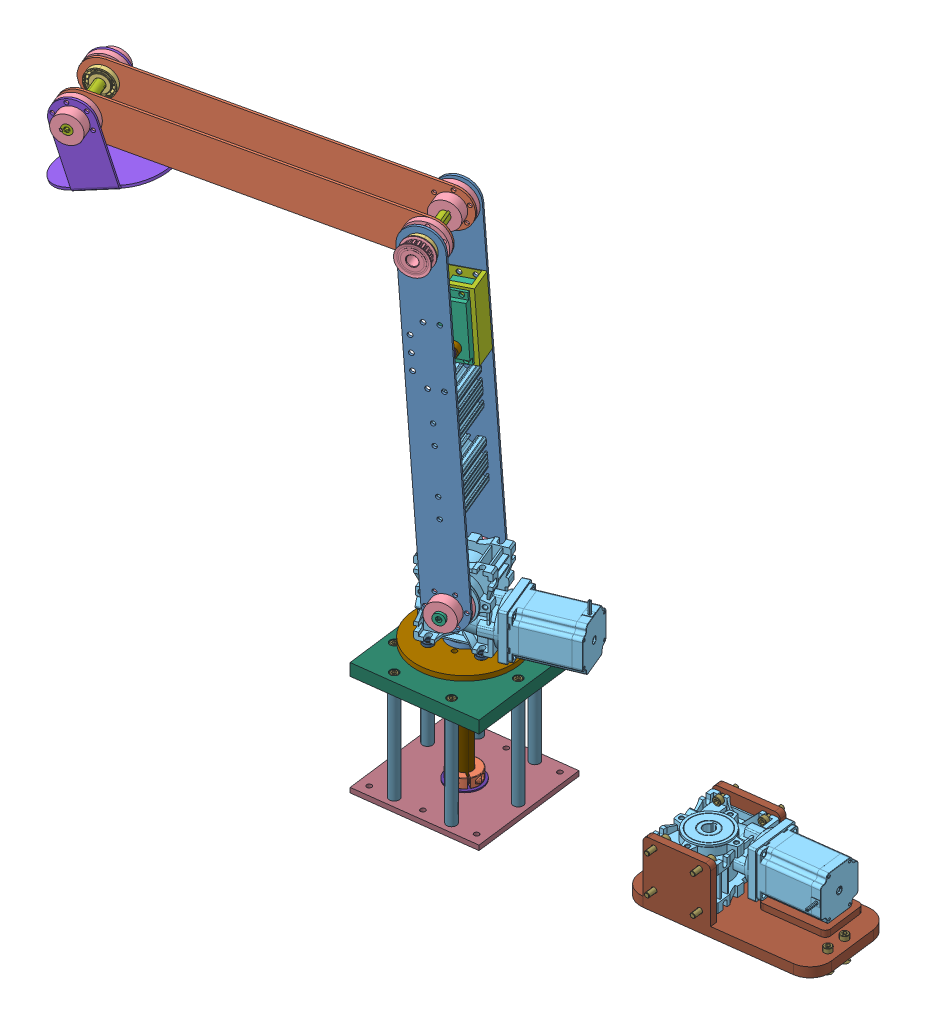
SolidWorks assembly Arm Assembly, configuration Default. Lengths in mm.
Overall size (892.51 782.73 345.65).
75 component instances, 30 part files, 141 mates.
Components (placement in the parent):
- Link 2-1: Link 2 [Default] at (1.4555 309.9129 324.2552) x (-0.057253 0.998075 0.023842) z (0.384426 0 0.923156) size (457.2 50.8 3.17)
- Link 3-1: Link 3 [Default] at (-14.0638 739.0935 409.0348) x (-0.91364 0.143211 0.380463) z (0.384426 0 0.923156) size (406.4 50.8 3.17)
- Flanged Bearing-1: Flanged Bearing [Default] at (-362.4163 764.8812 497.4483) x (0.923156 0 -0.384426) z (0.384426 0 0.923156) size (38.1 38.1 12.7)
- Keyed hub-1: Keyed hub [Default] at (9.2342 308.3376 408.8803) x (0.510272 -0.833349 -0.21249) z (-0.769311 -0.552748 0.320361) size (50.8 25.4 50.8)
- Link 2-2: Link 2 [Default] at (35.6886 309.9129 406.4623) x (-0.057253 0.998075 0.023842) z (0.384426 0 0.923156) size (457.2 50.8 3.17)
- Link 3-2: Link 3 [Default] at (-35.4177 739.0935 357.7558) x (-0.91364 0.143211 0.380463) z (0.384426 0 0.923156) size (406.4 50.8 3.17)
- Flanged Bearing-2: Flanged Bearing [Default] at (-9.7324 713.9553 428.8986) x (-0.878921 0.30584 0.366005) z (0.384426 0 0.923156) size (38.1 38.1 12.7)
- Flanged Bearing-3: Flanged Bearing [Default] at (-342.3416 764.8812 545.6555) x (-0.852745 -0.383049 0.355105) z (-0.384426 0 -0.923156) size (38.1 38.1 12.7)
- Keyed hub-2: Keyed hub [Default] at (-41.8271 713.9553 351.8267) x (0.725133 -0.618871 -0.301964) z (-0.571314 -0.785493 0.23791) size (50.8 25.4 50.8)
- Keyed hub-3: Keyed hub [Default] at (-17.6756 308.3376 344.2594) x (-0.510272 0.833349 0.21249) z (-0.769311 -0.552748 0.320361) size (50.8 25.4 50.8)
- Keyed hub-4: Keyed hub [Default] at (-13.1499 713.9553 420.6917) x (-0.725133 0.618871 0.301964) z (-0.571314 -0.785493 0.23791) size (50.8 25.4 50.8)
- Flanged Bearing-4: Flanged Bearing [Default] at (-45.2446 713.9553 343.6198) x (0.850075 0.38995 -0.353993) z (-0.384426 0 -0.923156) size (38.1 38.1 12.7)
- Nema Stepper Motor-2: Nema Stepper Motor [Default] at (64.8327 289.3684 347.8143) x (0.923156 0 -0.384426) z (-0.384426 0 -0.923156) size (171.01 100.01 63.01)
- Keyed Drive Shaft-1: Keyed Drive Shaft [Default] at (-50.3021 308.1752 256.2107) x (0.510272 -0.833349 -0.21249) z (0.384426 0 0.923156) size (19.9 19.9 128.01)
- Keyed Shaft-1: Keyed Shaft [Default] at (-51.2311 713.9553 329.2439) x (0.725133 -0.618871 -0.301964) z (0.384426 0 0.923156) size (12.7 12.5 104.14)
- Link 4-1: Link 4 [Default] at (-352.9478 683.5388 522.7917) x (0.384426 0 0.923156) z (-0.879568 -0.303649 0.366275) size (90.37 102.6 133.86)
- Keyed hub-5: Keyed hub [Default] at (-365.122 764.8812 490.9509) x (0.280315 -0.952784 -0.11673) z (0.879568 0.303649 -0.366275) size (50.8 25.4 50.8)
- Keyed hub-6: Keyed hub [Default] at (-338.9241 764.8812 553.8623) x (-0.280315 0.952784 0.11673) z (0.879568 0.303649 -0.366275) size (50.8 25.4 50.8)
- Keyed Shaft-2: Keyed Shaft [Default] at (-325.2539 764.8812 586.6897) x (0.280315 -0.952784 -0.11673) z (-0.384426 0 -0.923156) size (12.7 12.5 104.14)
- Joint 2 Motor Plate-1: Joint 2 Motor Plate [Default] at (-4.244 240.9876 376.7854) x (0.927827 0 0.373012) z (-0.373012 0 0.927827) size (127 6.35 127)
- 4 mm M6 spacer-1: 4 mm M6 spacer [94669A162] at (29.9074 249.3376 388.5617) x (-0.888418 0 -0.459036) z (0 -1 0) size (13 13 4)
- 4 mm M6 spacer-2: 4 mm M6 spacer [94669A162] at (-19.943 249.3376 409.3207) x (0.999963 0 0.008554) z (0 -1 0) size (13 13 4)
- 4 mm M6 spacer-3: 4 mm M6 spacer [94669A162] at (11.455 249.3376 344.2502) x (1 0 0) z (0 -1 0) size (13 13 4)
- 4 mm M6 spacer-4: 4 mm M6 spacer [94669A162] at (-38.3955 249.3376 365.0092) x (1 0 0) z (0 -1 0) size (13 13 4)
- Motor Mount Joint 1 Assembly-1: Motor Mount Joint 1 Assembly [Default] at (255.7253 -1.2672 148.6448) x (0.992107 0 -0.125391) z (0.125391 0 0.992107) size (228.6 94.85 140.08)
  - Joint 1 Motor Holder Bracket-1: Joint 1 Motor Holder Bracket [Default] at (55.8829 79.1234 191.166) size (228.6 82.55 114.78)
  - Nema Stepper Motor-1: Nema Stepper Motor [Default] at (81.7887 128.4828 180.6968) x (1 0 0) z (0 1 0) size (171.01 100.01 63.01)
  - Flanged Bearing-1: Flanged Bearing [Default] at (6.9829 88.5722 199.666) x (0.99323 0 0.116162) z (0 -1 0) size (38.1 38.1 12.7)
  - socket head cap screw_am-7: socket head cap screw_am [B18.3.1M - 6 x 1.0 x 25 Hex SHCS -- 25NHX] at (-20.0631 152.4828 153.666) x (0 0 -1) z (0.990069 0.140585 0) size (31 10 10)
  - socket head cap screw_am-8: socket head cap screw_am [B18.3.1M - 6 x 1.0 x 25 Hex SHCS -- 25NHX] at (33.9369 152.4828 228.666) x (0 0 1) z (-1 0 0) size (31 10 10)
  - socket head cap screw_am-9: socket head cap screw_am [B18.3.1M - 6 x 1.0 x 25 Hex SHCS -- 25NHX] at (-20.0631 152.4828 228.666) x (0 0 1) z (0.381849 0.924225 0) size (31 10 10)
  - socket head cap screw_am-10: socket head cap screw_am [B18.3.1M - 6 x 1.0 x 25 Hex SHCS -- 25NHX] at (-20.0631 104.4828 153.666) x (0 0 -1) z (0.756248 0.654286 0) size (31 10 10)
  - socket head cap screw_am-11: socket head cap screw_am [B18.3.1M - 6 x 1.0 x 25 Hex SHCS -- 25NHX] at (33.9369 104.4828 150.5881) x (0 0 -1) z (0.923728 0.383049 0) size (31 10 10)
  - socket head cap screw_am-12: socket head cap screw_am [B18.3.1M - 6 x 1.0 x 25 Hex SHCS -- 25NHX] at (-45.7171 97.8234 212.366) x (0 -1 0) z (-0.546944 0 0.837169) size (31 10 10)
  - socket head cap screw_am-19: socket head cap screw_am [B18.3.1M - 6 x 1.0 x 25 Hex SHCS -- 25NHX] at (-45.7171 97.8234 186.966) x (0 -1 0) z (-0.546944 0 0.837169) size (31 10 10)
  - socket head cap screw_am-14: socket head cap screw_am [B18.3.1M - 6 x 1.0 x 25 Hex SHCS -- 25NHX] at (33.9369 152.4828 153.666) x (0 0 -1) z (0.923728 0.383049 0) size (31 10 10)
  - socket head cap screw_am-15: socket head cap screw_am [B18.3.1M - 6 x 1.0 x 25 Hex SHCS -- 25NHX] at (157.4829 97.8234 186.966) x (0 -1 0) z (-0.546944 0 0.837169) size (31 10 10)
  - socket head cap screw_am-16: socket head cap screw_am [B18.3.1M - 6 x 1.0 x 25 Hex SHCS -- 25NHX] at (-20.0631 104.4828 228.666) x (0 0 1) z (-1 0 0) size (31 10 10)
  - socket head cap screw_am-17: socket head cap screw_am [B18.3.1M - 6 x 1.0 x 25 Hex SHCS -- 25NHX] at (33.9369 104.4828 228.666) x (0 0 1) z (-1 0 0) size (31 10 10)
  - socket head cap screw_am-18: socket head cap screw_am [B18.3.1M - 6 x 1.0 x 25 Hex SHCS -- 25NHX] at (157.4829 97.8234 212.366) x (0 -1 0) z (-0.546944 0 0.837169) size (31 10 10)
- Joint 1 bottom plate-1: Joint 1 bottom plate [89155K113] at (-4.244 81.0311 376.7854) x (-0.125391 0 -0.992107) z (0.992107 0 -0.125391) size (152.4 6.35 152.4)
- Base post-1: Base post [8974K269] at (21.393 160.4061 309.54) x (-0.837169 0 -0.546944) z (0 -1 0) size (12.7 12.7 127)
- Base post-2: Base post [8974K269] at (-29.8811 160.4061 444.0308) x (-0.837169 0 -0.546944) z (0 -1 0) size (12.7 12.7 127)
- Base post-3: Base post [8974K269] at (37.3177 160.4061 435.5376) x (0.463623 0 0.886032) z (0 -1 0) size (12.7 12.7 127)
- Base post-4: Base post [8974K269] at (58.7548 160.4061 368.8231) x (-0.837169 0 -0.546944) z (0 -1 0) size (12.7 12.7 127)
- Base post-5: Base post [8974K269] at (-70.4278 160.4061 359.5483) x (-0.837169 0 -0.546944) z (0 -1 0) size (12.7 12.7 127)
- Base post-6: Base post [8974K269] at (-45.8058 160.4061 318.0332) x (-0.837169 0 -0.546944) z (0 -1 0) size (12.7 12.7 127)
- Base post-7: Base post [8974K269] at (-64.0579 160.4061 409.9473) x (-0.837169 0 -0.546944) z (0 -1 0) size (12.7 12.7 127)
- Joint 1 top plate-1: Joint 1 top plate [89155K143] at (-4.244 219.1436 376.7854) x (-0.125391 0 -0.992107) z (0.992107 0 -0.125391) size (152.4 15.88 152.4)
- Tapered-Roller Bearing-1: Tapered-Roller Bearing [5709K77] at (-4.244 223.5886 376.7854) x (1 0 0) z (0 -1 0) size (45.24 45.24 17.1)
- base Ball Bearing 0.75 in-1: base Ball Bearing 0.75 in [6384K367] at (-4.244 79.4436 376.7854) x (1 0 0) z (0 -1 0) size (44.45 44.45 14.27)
- keyed shaft 0.75 in bore 9 in-1: keyed shaft 0.75 in bore 9 in [Default] at (-4.244 140.9751 376.7854) x (0.927827 0 0.373012) z (0 -1 0) size (19.05 18.75 228.6)
- 0.75 in shaft hub-1: 0.75 in shaft hub [Default] at (-4.244 234.6376 376.7854) x (-0.927827 0 -0.373012) z (0 -1 0) size (63.5 63.5 19.49)
- Clamping Two-Piece Shaft Collar 0.75 in-1: Clamping Two-Piece Shaft Collar 0.75 in [6436K16] at (-4.244 92.1436 376.7854) x (0.845517 0 0.533948) z (0 1 0) size (38.06 38.1 12.77)
- T-slot Slider-1: T-slot Slider [5278N52] at (236.9979 67.7205 365.0672) x (-0.837169 0 -0.546944) z (0 1 0) size (10 9.8 4.82)
- T-slot Slider-2: T-slot Slider [5278N52] at (233.8129 65.4156 339.8677) x (-0.837169 0 -0.546944) z (0 1 0) size (10 9.8 4.82)
- T-slot Slider-3: T-slot Slider [5278N52] at (438.5941 68.7454 339.5877) x (-0.838988 0 -0.544149) z (0 1 0) size (10 9.8 4.82)
- T-slot Slider-4: T-slot Slider [5278N52] at (435.4091 66.889 314.3882) x (-0.837169 0 -0.546944) z (0 1 0) size (10 9.8 4.82)
- joint3pulley-1: joint3pulley [6495K752] at (-5.8985 713.9553 438.1053) x (0.86916 -0.336987 -0.36194) z (-0.384426 0 -0.923156) size (38.1 38.1 22.23)
- 8020tframeforjoint3-1: 8020tframeforjoint3 [47065T653] at (-23.5517 422.4176 348.5885) x (0.921379 0.062019 -0.383686) z (0.384426 0 0.923156) size (25.4 50.8 85.85)
- 8020tframeforjoint3-2: 8020tframeforjoint3 [47065T653] at (-28.285 504.9314 350.5596) x (0.921379 0.062019 -0.383686) z (0.384426 0 0.923156) size (25.4 50.8 85.85)
- 80 kg-1: 80 kg [Default] at (-47.5369 625.3222 348.9217) x (0.057253 -0.998075 -0.023842) z (-0.921379 -0.062019 0.383686) size (82 48 30)
- servobracket_80kg-1: servobracket_80kg [Default] at (-37.0502 593.4851 343.7293) x (0.057253 -0.998075 -0.023842) z (-0.921379 -0.062019 0.383686) size (87.12 31.24 59.67)
- 3422-0004-0020 assembly.STEP-1: 3422-0004-0020 assembly.STEP [Default] at (13.1466 564.3048 357.8431) x (0.821772 -0.455616 -0.342207) z (-0.420604 -0.890177 0.17515) size (15 18 15.01)
  - 3422-0004-0020 core.STEP-1: 3422-0004-0020 core.STEP [Default] at (-35.1952 21.4358 6.7264) size (12.22 18 12.22)
  - 3422 series barrel.STEP-1: 3422 series barrel.STEP [Default] at (-35.1952 8.9358 6.7264) x (1 0 0) z (0 1 0) size (15 15.01 9)
  - 3422 series flange.STEP-1: 3422 series flange.STEP [Default] at (-35.1952 24.9358 6.7264) x (1 0 0) z (0 1 0) size (15 15 1)
  - 2806-0005-0005_91390A117.STEP-1: 2806-0005-0005_91390A117.STEP [Default] at (-35.1952 13.4358 11.638) x (-0.412538 -0.91094 0) z (0 0 1) size (5.01 5.01 5.01)
- socket head cap screw_ai-1: socket head cap screw_ai [HX-SHCS 0.25-20x1.5x1-N] at (-29.8811 227.0811 444.0308) x (0 -1 0) z (0 0 1) size (44.45 9.53 9.53)
- socket head cap screw_ai-2: socket head cap screw_ai [HX-SHCS 0.25-20x1.5x1-N] at (-70.4278 227.0811 359.5483) x (0 -1 0) z (0 0 1) size (44.45 9.53 9.53)
- socket head cap screw_ai-3: socket head cap screw_ai [HX-SHCS 0.25-20x1.5x1-N] at (-64.0579 227.0811 409.9473) x (0 -1 0) z (0 0 1) size (44.45 9.53 9.53)
- socket head cap screw_ai-4: socket head cap screw_ai [HX-SHCS 0.25-20x1.5x1-N] at (21.393 227.0811 309.54) x (0 -1 0) z (-0.556107 0 0.831111) size (44.45 9.53 9.53)
- socket head cap screw_ai-5: socket head cap screw_ai [HX-SHCS 0.25-20x1.5x1-N] at (-45.8058 227.0811 318.0332) x (0 -1 0) z (0 0 1) size (44.45 9.53 9.53)
- socket head cap screw_ai-6: socket head cap screw_ai [HX-SHCS 0.25-20x1.5x1-N] at (58.7548 227.0811 368.8231) x (0 -1 0) z (0 0 1) size (44.45 9.53 9.53)
- socket head cap screw_ai-7: socket head cap screw_ai [HX-SHCS 0.25-20x1.5x1-N] at (37.3177 227.0811 435.5376) x (0 -1 0) z (0 0 1) size (44.45 9.53 9.53)
Mates (geometry in assembly coordinates):
- Concentric3: concentric aligned: cylinder of Keyed hub-1 through (12.2856 308.3376 416.2079) axis (0.384426 0 0.923156) radius 17.4625; cylinder of Link 2-2 through (12.2856 308.3376 416.2079) axis (0.384426 0 0.923156) radius 17.4625
- Coincident2: coincident anti-aligned: plane of Keyed hub-1 through (12.2856 308.3376 416.2079) normal (0.384426 0 0.923156); plane of Link 2-2 through (12.2856 308.3376 416.2079) normal (-0.384426 0 -0.923156)
- Concentric4: concentric aligned: cylinder of Keyed hub-1 through (23.0431 290.769 411.7282) axis (0.384426 0 0.923156) radius 2.5527; cylinder of Link 2-2 through (24.2637 290.769 414.6592) axis (0.384426 0 0.923156) radius 2.5527
- Concentric5: concentric anti-aligned: cylinder of Link 2-1 through (-21.9475 308.3376 334.0009) axis (0.384426 0 0.923156) radius 17.4625; cylinder of Keyed hub-3 through (-20.727 308.3376 336.9319) axis (-0.384426 0 -0.923156) radius 17.4625
- Coincident3: coincident anti-aligned: plane of Link 2-1 through (-20.727 308.3376 336.9319) normal (0.384426 0 0.923156); plane of Keyed hub-3 through (-20.727 308.3376 336.9319) normal (-0.384426 0 -0.923156)
- Concentric7: concentric anti-aligned: cylinder of Link 2-1 through (-40.1515 307.0302 345.0207) axis (0.384426 0 0.923156) radius 2.5527; cylinder of Keyed hub-3 through (-40.1515 307.0302 345.0207) axis (-0.384426 0 -0.923156) radius 2.5527
- Concentric8: concentric anti-aligned: cylinder of Keyed hub-1 through (9.2342 308.3376 408.8803) axis (0.384426 0 0.923156) radius 6.35; cylinder of Keyed hub-3 through (-17.6756 308.3376 344.2594) axis (-0.384426 0 -0.923156) radius 6.35
- Coincident5: coincident aligned: plane of Keyed hub-1 through (8.4241 309.6606 409.2177) normal (0.510272 -0.833349 -0.21249); plane of Keyed hub-3 through (-18.4857 309.6606 344.5968) normal (0.510272 -0.833349 -0.21249)
- Concentric9: concentric aligned: cylinder of Link 2-2 through (-10.9822 713.9553 425.8972) axis (0.384426 0 0.923156) radius 17.4625; cylinder of Flanged Bearing-2 through (-7.2913 713.9553 434.7606) axis (0.384426 0 0.923156) radius 17.4625
- Concentric10: concentric anti-aligned: cylinder of Link 2-1 through (-45.2153 713.9553 343.6902) axis (0.384426 0 0.923156) radius 17.4625; cylinder of Flanged Bearing-4 through (-47.6857 713.9553 337.7578) axis (-0.384426 0 -0.923156) radius 17.4625
- Concentric11: concentric anti-aligned: cylinder of Link 3-1 through (-17.4218 713.9553 410.4331) axis (0.384426 0 0.923156) radius 17.4625; cylinder of Keyed hub-4 through (-16.2013 713.9553 413.3642) axis (-0.384426 0 -0.923156) radius 17.4625
- Coincident8: coincident anti-aligned: plane of Link 3-1 through (-16.2013 713.9553 413.3642) normal (0.384426 0 0.923156); plane of Keyed hub-4 through (-16.2013 713.9553 413.3642) normal (-0.384426 0 -0.923156)
- Concentric12: concentric anti-aligned: cylinder of Link 3-1 through (-13.4141 734.82 412.2035) axis (0.384426 0 0.923156) radius 2.5527; cylinder of Keyed hub-4 through (-13.4141 734.82 412.2035) axis (-0.384426 0 -0.923156) radius 2.5527
- Concentric13: concentric aligned: cylinder of Link 3-2 through (-38.7757 713.9553 359.1542) axis (0.384426 0 0.923156) radius 17.4625; cylinder of Keyed hub-2 through (-38.7757 713.9553 359.1542) axis (0.384426 0 0.923156) radius 17.4625
- Coincident9: coincident anti-aligned: plane of Link 3-2 through (-38.7757 713.9553 359.1542) normal (-0.384426 0 -0.923156); plane of Keyed hub-2 through (-38.7757 713.9553 359.1542) normal (0.384426 0 0.923156)
- Concentric14: concentric aligned: cylinder of Link 3-2 through (-34.768 734.82 360.9246) axis (0.384426 0 0.923156) radius 2.5527; cylinder of Keyed hub-2 through (-35.9885 734.82 357.9936) axis (0.384426 0 0.923156) radius 2.5527
- Concentric15: concentric anti-aligned: cylinder of Keyed hub-2 through (-41.8271 713.9553 351.8267) axis (0.384426 0 0.923156) radius 6.35; cylinder of Keyed hub-4 through (-13.1499 713.9553 420.6917) axis (-0.384426 0 -0.923156) radius 6.35
- Coincident10: coincident aligned: plane of Keyed hub-2 through (-40.6759 712.9729 351.3473) normal (-0.725133 0.618871 0.301964); plane of Keyed hub-4 through (-11.9988 712.9729 420.2123) normal (-0.725133 0.618871 0.301964)
- Concentric16: concentric aligned: cylinder of Flanged Bearing-2 through (-7.2913 713.9553 434.7606) axis (0.384426 0 0.923156) radius 6.35; cylinder of Keyed hub-2 through (-41.8271 713.9553 351.8267) axis (0.384426 0 0.923156) radius 6.35
- Concentric17: concentric aligned: cylinder of Flanged Bearing-1 through (-359.9752 764.8812 503.3103) axis (0.384426 0 0.923156) radius 17.4625; cylinder of Link 3-2 through (-363.6661 764.8812 494.4469) axis (0.384426 0 0.923156) radius 17.4625
- Coincident13: coincident anti-aligned: plane of Flanged Bearing-1 through (-363.6661 782.3437 494.4469) normal (0.384426 0 0.923156); plane of Link 3-2 through (-38.7757 713.9553 359.1542) normal (-0.384426 0 -0.923156)
- Concentric18: concentric anti-aligned: cylinder of Link 3-1 through (-342.3123 764.8812 545.7258) axis (0.384426 0 0.923156) radius 17.4625; cylinder of Flanged Bearing-3 through (-344.7827 764.8812 539.7934) axis (-0.384426 0 -0.923156) radius 17.4625
- Coincident14: coincident anti-aligned: plane of Link 3-1 through (-16.2013 713.9553 413.3642) normal (0.384426 0 0.923156); plane of Flanged Bearing-3 through (-347.2667 781.0118 551.2282) normal (-0.384426 0 -0.923156)
- Concentric21: concentric anti-aligned: cylinder of Keyed hub-1 through (9.2342 308.3376 408.8803) axis (0.384426 0 0.923156) radius 6.35; cylinder of Keyed Drive Shaft-1 through (20.3825 308.3376 435.6519) axis (-0.384426 0 -0.923156) radius 7
- Parallel1: parallel anti-aligned: plane of Keyed hub-1 through (8.4241 309.6606 409.2177) normal (0.510272 -0.833349 -0.21249); plane of Keyed Drive Shaft-1 through (-1.419 313.3506 375.4032) normal (-0.510272 0.833349 0.21249)
- Coincident18: coincident anti-aligned: plane of Keyed hub-3 through (-17.6756 308.3376 344.2594) normal (0.384426 0 0.923156); plane of Keyed Drive Shaft-1 through (-13.1387 313.0374 342.3702) normal (-0.384426 0 -0.923156)
- Coincident19: coincident anti-aligned: plane of Keyed hub-1 through (9.2342 308.3376 408.8803) normal (-0.384426 0 -0.923156); plane of Keyed Drive Shaft-1 through (13.7711 313.0374 406.9911) normal (0.384426 0 0.923156)
- Concentric22: concentric anti-aligned: cylinder of Keyed hub-2 through (-41.8271 713.9553 351.8267) axis (0.384426 0 0.923156) radius 6.35; cylinder of Keyed Shaft-1 through (-7.2913 713.9553 434.7606) axis (-0.384426 0 -0.923156) radius 6.35
- Coincident20: coincident aligned: plane of Keyed hub-2 through (-40.6759 712.9729 351.3473) normal (-0.725133 0.618871 0.301964); plane of Keyed Shaft-1 through (-3.4265 716.7038 433.1512) normal (-0.725133 0.618871 0.301964)
- Coincident22: coincident anti-aligned: plane of Link 2-1 through (-20.727 308.3376 336.9319) normal (0.384426 0 0.923156); plane of Flanged Bearing-4 through (-37.7085 697.8752 344.0034) normal (-0.384426 0 -0.923156)
- Distance1: distance = 2.54 mm anti-aligned: plane of Flanged Bearing-4 through (-38.6614 703.36 347.757) normal (0.384426 0 0.923156); plane of Keyed hub-2 through (-41.8271 713.9553 351.8267) normal (-0.384426 0 -0.923156)
- Coincident24: coincident anti-aligned: plane of Link 2-2 through (12.2856 308.3376 416.2079) normal (-0.384426 0 -0.923156); plane of Flanged Bearing-2 through (-15.9125 697.3296 427.9503) normal (0.384426 0 0.923156)
- Distance2: distance = 2.54 mm anti-aligned: plane of Keyed hub-4 through (-13.1499 713.9553 420.6917) normal (0.384426 0 0.923156); plane of Flanged Bearing-2 through (-15.4221 703.0004 424.3893) normal (-0.384426 0 -0.923156)
- Coincident26: coincident aligned: plane of Flanged Bearing-2 through (-9.0841 707.9096 435.5072) normal (0.384426 0 0.923156); plane of Keyed Shaft-1 through (-7.2913 713.9553 434.7606) normal (0.384426 0 0.923156)
- Concentric23: concentric anti-aligned: cylinder of Link 4-1 through (-334.6521 764.8812 564.1209) axis (-0.384426 0 -0.923156) radius 17.4625; cylinder of Keyed hub-6 through (-335.8727 764.8812 561.1899) axis (0.384426 0 0.923156) radius 17.4625
- Concentric24: concentric anti-aligned: cylinder of Link 4-1 through (-354.8862 769.3806 569.1076) axis (-0.384426 0 -0.923156) radius 2.5527; cylinder of Keyed hub-6 through (-354.8862 769.3806 569.1076) axis (0.384426 0 0.923156) radius 2.5527
- Coincident27: coincident anti-aligned: plane of Link 4-1 through (-325.3006 644.4612 556.7874) normal (-0.384426 0 -0.923156); plane of Keyed hub-6 through (-335.8727 764.8812 561.1899) normal (0.384426 0 0.923156)
- Concentric25: concentric anti-aligned: cylinder of Link 4-1 through (-369.3939 764.8812 480.6923) axis (0.384426 0 0.923156) radius 17.4625; cylinder of Keyed hub-5 through (-368.1733 764.8812 483.6233) axis (-0.384426 0 -0.923156) radius 17.4625
- Concentric26: concentric anti-aligned: cylinder of Link 4-1 through (-387.1869 769.3806 491.5411) axis (0.384426 0 0.923156) radius 2.5527; cylinder of Keyed hub-5 through (-387.1869 769.3806 491.5411) axis (-0.384426 0 -0.923156) radius 2.5527
- Concentric27: concentric anti-aligned: cylinder of Keyed hub-5 through (-365.122 764.8812 490.9509) axis (-0.384426 0 -0.923156) radius 6.35; cylinder of Keyed Shaft-2 through (-369.1937 764.8812 481.173) axis (0.384426 0 0.923156) radius 6.35
- Coincident31: coincident aligned: plane of Keyed hub-5 through (-365.567 766.3937 491.1362) normal (0.280315 -0.952784 -0.11673); plane of Keyed Shaft-2 through (-373.8165 764.9514 483.0981) normal (0.280315 -0.952784 -0.11673)
- Coincident32: coincident aligned: plane of Keyed hub-6 through (-329.1596 764.8812 577.3105) normal (0.384426 0 0.923156); plane of Keyed Shaft-2 through (-329.1596 764.8812 577.3105) normal (0.384426 0 0.923156)
- Coincident34: coincident anti-aligned: plane of Link 4-1 through (-357.6013 644.4612 479.2209) normal (0.384426 0 0.923156); plane of Keyed hub-5 through (-368.1733 764.8812 483.6233) normal (-0.384426 0 -0.923156)
- Coincident36: coincident aligned: plane of Keyed hub-6 through (-338.4791 763.3686 553.677) normal (-0.280315 0.952784 0.11673); plane of Keyed Shaft-2 through (-372.9265 761.9264 482.7274) normal (-0.280315 0.952784 0.11673)
- Concentric28: concentric anti-aligned: cone of Flanged Bearing-3 through (-340.1579 764.8812 550.8993) axis (-0.384426 0 -0.923156); cylinder of Keyed Shaft-2 through (-369.1937 764.8812 481.173) axis (0.384426 0 0.923156) radius 6.35
- Distance3: distance = 2.54 mm anti-aligned: plane of Flanged Bearing-3 through (-343.9692 775.5098 553.2118) normal (0.384426 0 0.923156); plane of Keyed hub-6 through (-338.9241 764.8812 553.8623) normal (-0.384426 0 -0.923156)
- Coincident38: coincident anti-aligned: plane of Top base plate-1 through (74.0847 244.0001 261.2257) normal (0 -1 0); plane of arm base spacer small part-1 through (130.8381 244.0001 364.6329) normal (0 1 0)
- Coincident40: coincident anti-aligned: plane of Top base plate-1 through (74.0847 244.0001 261.2257) normal (0 -1 0); plane of arm base spacer large part-1 through (32.1724 244.0001 346.1862) normal (0 1 0)
- Coincident45: coincident anti-aligned: plane of Bearing other part-1 through (32.1724 247.1751 346.1862) normal (0 -1 0); plane of Top base plate-1 through (74.0847 247.1751 261.2257) normal (0 1 0)
- Concentric32: concentric aligned: cylinder of Bearing other part-1 through (32.1724 257.1751 346.1862) axis (0 -1 0) radius 70; circle of arm base spacer large part-1
- Coincident57: coincident aligned: plane of Top base plate-1 through (-6.0476 247.1751 446.2586) normal (0.059501 0 0.998228); plane of arm base spacer large part-1 through (84.7912 244.0001 440.844) normal (0.059501 0 0.998228)
- Coincident58: coincident aligned: plane of Top base plate-1 through (-75.7951 247.1751 376.9496) normal (-0.998228 0 0.059501); plane of arm base spacer large part-1 through (-75.8042 244.0001 376.7975) normal (-0.998228 0 0.059501)
- Concentric37: concentric aligned: cylinder of Top base plate-1 through (130.8381 247.1751 364.6329) axis (0 -1 0) radius 15; cylinder of arm base spacer small part-1 through (130.8381 244.0001 364.6329) axis (0 -1 0) radius 15
- Coincident59: coincident aligned: plane of Top base plate-1 through (145.8116 247.1751 363.7404) normal (0.998228 0 -0.059501); plane of arm base spacer small part-1 through (145.8116 244.0001 363.7404) normal (0.998228 0 -0.059501)
- Parallel2: parallel aligned: plane of Nema Stepper Motor-3 through (350.3499 203.0272 320.7095) normal (0 1 0); plane of Top base plate-1 through (74.0847 247.1751 261.2257) normal (0 1 0)
- Parallel3: parallel anti-aligned: plane of Nema Stepper Motor-3 through (312.2058 175.0272 353.0364) normal (-0.998228 0 0.059501); plane of arm base spacer small part-1 through (145.8116 244.0001 363.7404) normal (0.998228 0 -0.059501)
- Coincident61: coincident anti-aligned: plane of Nema Stepper Motor-2 through (43.4654 251.3376 387.0429) normal (0 -1 0); plane of 4 mm M6 spacer-1 through (29.9074 251.3376 388.5617) normal (0 1 0)
- Concentric43: concentric aligned: cylinder of Keyed hub-1 through (12.2856 308.3376 416.2079) axis (0.384426 0 0.923156) radius 17.4625; cylinder of Nema Stepper Motor-2 through (-39.8667 308.3376 290.9699) axis (0.384426 0 0.923156) radius 7
- Coincident65: coincident anti-aligned: plane of Nema Stepper Motor-2 through (7.8846 308.3376 405.651) normal (0.384426 0 0.923156); plane of Keyed Drive Shaft-1 through (7.8887 308.3376 405.6493) normal (-0.384426 0 -0.923156)
- Concentric44: concentric aligned: cylinder of Joint 1 bottom plate-1 through (58.7548 83.9521 368.8231) axis (0 1 0) radius 1.905; cylinder of Base post-4 through (58.7548 84.2061 368.8231) axis (0 1 0) radius 6.35
- Concentric45: concentric aligned: cylinder of Joint 1 bottom plate-1 through (37.3177 83.9521 435.5376) axis (0 1 0) radius 1.905; cylinder of Base post-3 through (37.3177 84.2061 435.5376) axis (0 1 0) radius 6.35
- Concentric46: concentric aligned: cylinder of Joint 1 bottom plate-1 through (-29.8811 83.9521 444.0308) axis (0 1 0) radius 1.905; cylinder of Base post-2 through (-29.8811 84.2061 444.0308) axis (0 1 0) radius 6.35
- Concentric47: concentric aligned: cylinder of Joint 1 bottom plate-1 through (21.393 83.9521 309.54) axis (0 1 0) radius 1.905; cylinder of Base post-1 through (21.393 84.2061 309.54) axis (0 1 0) radius 6.35
- Concentric48: concentric aligned: cylinder of Joint 1 bottom plate-1 through (-45.8058 83.9521 318.0332) axis (0 1 0) radius 1.905; cylinder of Base post-6 through (-45.8058 84.2061 318.0332) axis (0 1 0) radius 6.35
- Concentric49: concentric aligned: cylinder of Joint 1 bottom plate-1 through (-64.0579 83.9521 409.9473) axis (0 1 0) radius 1.905; cylinder of Base post-7 through (-64.0579 84.2061 409.9473) axis (0 1 0) radius 6.35
- Concentric50: concentric aligned: cylinder of Joint 1 bottom plate-1 through (-70.4278 83.9521 359.5483) axis (0 1 0) radius 1.905; cylinder of Base post-5 through (-70.4278 84.2061 359.5483) axis (0 1 0) radius 6.35
- Coincident66: coincident anti-aligned: plane of Joint 1 bottom plate-1 through (80.9094 84.2061 442.8292) normal (0 1 0); plane of Base post-4 through (58.7548 84.2061 368.8231) normal (0 -1 0)
- Coincident67: coincident anti-aligned: plane of Joint 1 bottom plate-1 through (80.9094 84.2061 442.8292) normal (0 1 0); plane of Base post-3 through (37.3177 84.2061 435.5376) normal (0 -1 0)
- Coincident68: coincident anti-aligned: plane of Joint 1 bottom plate-1 through (80.9094 84.2061 442.8292) normal (0 1 0); plane of Base post-2 through (-29.8811 84.2061 444.0308) normal (0 -1 0)
- Coincident69: coincident anti-aligned: plane of Joint 1 bottom plate-1 through (80.9094 84.2061 442.8292) normal (0 1 0); plane of Base post-7 through (-64.0579 84.2061 409.9473) normal (0 -1 0)
- Coincident70: coincident anti-aligned: plane of Joint 1 bottom plate-1 through (80.9094 84.2061 442.8292) normal (0 1 0); plane of Base post-1 through (21.393 84.2061 309.54) normal (0 -1 0)
- Coincident71: coincident anti-aligned: plane of Joint 1 bottom plate-1 through (80.9094 84.2061 442.8292) normal (0 1 0); plane of Base post-6 through (-45.8058 84.2061 318.0332) normal (0 -1 0)
- Coincident72: coincident anti-aligned: plane of Joint 1 bottom plate-1 through (80.9094 84.2061 442.8292) normal (0 1 0); plane of Base post-5 through (-70.4278 84.2061 359.5483) normal (0 -1 0)
- Coincident75: coincident anti-aligned: plane of Base post-3 through (37.3177 211.2061 435.5376) normal (0 1 0); plane of Joint 1 top plate-1 through (61.7997 211.2061 291.632) normal (0 -1 0)
- Parallel5: parallel aligned: plane of Motor Mount Joint 1 Assembly-1/Joint 1 Motor Holder Bracket-1 through (228.936 90.5561 402.5641) normal (0.125391 0 0.992107); plane of Joint 1 bottom plate-1 through (80.9094 77.8561 442.8292) normal (0.125391 0 0.992107)
- Coincident79: coincident anti-aligned: plane of Joint 1 top plate-1 through (-4.244 217.5561 376.7854) normal (0 1 0); plane of Tapered-Roller Bearing-1 through (-4.244 217.5561 399.4073) normal (0 -1 0)
- Concentric51: concentric anti-aligned: cylinder of Joint 1 top plate-1 through (-4.244 217.5561 376.7854) axis (0 1 0) radius 22.6219; cylinder of Tapered-Roller Bearing-1 through (-4.244 223.5886 376.7854) axis (0 -1 0) radius 22.6219
- Coincident80: coincident anti-aligned: plane of Nema Stepper Motor-2 through (43.4654 251.3376 387.0429) normal (0 -1 0); plane of 4 mm M6 spacer-2 through (-19.943 251.3376 409.3207) normal (0 1 0)
- Coincident81: coincident anti-aligned: plane of Nema Stepper Motor-2 through (43.4654 251.3376 387.0429) normal (0 -1 0); plane of 4 mm M6 spacer-4 through (-38.3955 251.3376 365.0092) normal (0 1 0)
- Concentric52: concentric anti-aligned: cylinder of Joint 1 bottom plate-1 through (-4.244 77.8561 376.7854) axis (0 1 0) radius 20.6375; cylinder of base Ball Bearing 0.75 in-1 through (-4.244 73.0936 376.7854) axis (0 -1 0) radius 20.6375
- Coincident82: coincident anti-aligned: plane of Joint 1 bottom plate-1 through (80.9094 84.2061 442.8292) normal (0 1 0); plane of base Ball Bearing 0.75 in-1 through (-4.244 84.2061 395.7927) normal (0 -1 0)
- Concentric53: concentric anti-aligned: cylinder of base Ball Bearing 0.75 in-1 through (-4.244 73.0936 376.7854) axis (0 -1 0) radius 9.525; cylinder of keyed shaft 0.75 in bore-1 through (-4.244 -126.3486 376.7854) axis (0 1 0) radius 9.525
- Concentric54: concentric anti-aligned: cylinder of base Ball Bearing 0.75 in-1 through (-4.244 73.0936 376.7854) axis (0 -1 0) radius 9.525; cylinder of keyed shaft 0.75 in bore 9 in-1 through (-4.244 26.6751 376.7854) axis (0 1 0) radius 9.525
- Coincident83: coincident aligned: plane of Motor Mount Joint 1 Assembly-1/Joint 1 Motor Holder Bracket-1 through (335.1377 77.8561 331.2948) normal (0 -1 0); plane of Joint 1 bottom plate-1 through (61.7997 77.8561 291.632) normal (0 -1 0)
- Concentric55: concentric aligned: cylinder of Joint 2 Motor Plate-1 through (-4.244 240.9876 376.7854) axis (0 1 0) radius 20.6375; circle of 0.75 in shaft hub-1
- Concentric56: concentric anti-aligned: cylinder of Joint 2 Motor Plate-1 through (-14.2088 240.9876 353.4217) axis (0 1 0) radius 3.175; circle of 0.75 in shaft hub-1
- Concentric57: concentric aligned: cylinder of keyed shaft 0.75 in bore 9 in-1 through (-4.244 26.6751 376.7854) axis (0 1 0) radius 9.525; cylinder of 0.75 in shaft hub-1 through (-4.244 233.0501 376.7854) axis (0 1 0) radius 9.525
- Parallel6: parallel aligned: plane of keyed shaft 0.75 in bore 9 in-1 through (-9.1217 26.6751 382.5171) normal (0.927827 0 0.373012); plane of 0.75 in shaft hub-1 through (-10.8946 234.6376 386.9441) normal (0.927827 0 0.373012)
- Coincident90: coincident anti-aligned: plane of Joint 2 Motor Plate-1 through (-4.244 240.9876 376.7854) normal (0 -1 0); plane of 0.75 in shaft hub-1 through (-4.244 240.9876 376.7854) normal (0 1 0)
- Concentric60: concentric anti-aligned: cylinder of keyed shaft 0.75 in bore 9 in-1 through (-4.244 26.6751 376.7854) axis (0 1 0) radius 9.525; cylinder of Clamping Two-Piece Shaft Collar 0.75 in-1 through (-4.244 98.4936 376.7854) axis (0 -1 0) radius 9.525
- Distance9: distance = 1.5875 mm aligned: plane of keyed shaft 0.75 in bore 9 in-1 through (-4.244 255.2751 376.7854) normal (0 1 0); plane of 0.75 in shaft hub-1 through (-4.244 253.6876 376.7854) normal (0 1 0)
- Coincident95: coincident anti-aligned: plane of Nema Stepper Motor-2 through (43.4654 251.3376 387.0429) normal (0 -1 0); plane of 4 mm M6 spacer-3 through (11.455 251.3376 344.2502) normal (0 1 0)
- Coincident96: coincident anti-aligned: plane of Joint 2 Motor Plate-1 through (-4.244 247.3376 376.7854) normal (0 1 0); plane of 4 mm M6 spacer-3 through (11.455 247.3376 344.2502) normal (0 -1 0)
- Concentric62: concentric anti-aligned: cylinder of Joint 2 Motor Plate-1 through (29.9074 240.9876 388.5617) axis (0 1 0) radius 3.25; cylinder of 4 mm M6 spacer-1 through (29.9074 251.3376 388.5617) axis (0 -1 0) radius 3.15
- Concentric63: concentric anti-aligned: cylinder of Joint 2 Motor Plate-1 through (-19.943 240.9876 409.3207) axis (0 1 0) radius 3.25; cylinder of 4 mm M6 spacer-2 through (-19.943 251.3376 409.3207) axis (0 -1 0) radius 3.15
- Tangent1: tangent anti-aligned: plane of Nema Stepper Motor-2 through (26.1576 274.039 387.7509) normal (0.923156 0 -0.384426); cylinder of 4 mm M6 spacer-1 through (29.9074 251.3376 388.5617) axis (0 -1 0) radius 3.15
- Tangent2: tangent anti-aligned: plane of Nema Stepper Motor-2 through (-23.6929 274.039 408.5099) normal (0.923156 0 -0.384426); cylinder of 4 mm M6 spacer-2 through (-19.943 251.3376 409.3207) axis (0 -1 0) radius 3.15
- Tangent3: tangent anti-aligned: plane of Nema Stepper Motor-2 through (9.2428 274.039 347.132) normal (0.923156 0 -0.384426); cylinder of 4 mm M6 spacer-3 through (11.455 251.3376 344.2502) axis (0 -1 0) radius 3.15
- Concentric67: concentric anti-aligned: cylinder of Joint 2 Motor Plate-1 through (-38.3955 240.9876 365.0092) axis (0 1 0) radius 3.25; cylinder of 4 mm M6 spacer-4 through (-38.3955 251.3376 365.0092) axis (0 -1 0) radius 3.15
- Tangent5: tangent anti-aligned: plane of Nema Stepper Motor-2 through (-40.6076 274.039 367.891) normal (0.923156 0 -0.384426); cylinder of 4 mm M6 spacer-4 through (-38.3955 251.3376 365.0092) axis (0 -1 0) radius 3.15
- Concentric68: concentric anti-aligned: cylinder of Joint 2 Motor Plate-1 through (11.455 240.9876 344.2502) axis (0 1 0) radius 3.25; cylinder of 4 mm M6 spacer-3 through (11.455 251.3376 344.2502) axis (0 -1 0) radius 3.15
- Distance11: distance = 3.81 mm: point of 4 mm M6 spacer-1; plane of Nema Stepper Motor-2 through (6.5392 308.3376 402.4199) normal (0.384426 0 0.923156)
- Concentric69: concentric aligned: cylinder of Motor Mount Joint 1 Assembly-1/socket head cap screw_am-18 through (438.5941 128.3061 339.5877) axis (0 1 0) radius 3; circle of T-slot Slider-3
- Concentric70: concentric aligned: cylinder of Motor Mount Joint 1 Assembly-1/socket head cap screw_am-15 through (435.4091 128.3061 314.3882) axis (0 1 0) radius 3; circle of T-slot Slider-4
- Concentric71: concentric aligned: cylinder of Motor Mount Joint 1 Assembly-1/socket head cap screw_am-12 through (236.9979 128.3061 365.0672) axis (0 1 0) radius 3; circle of T-slot Slider-1
- Concentric72: concentric aligned: cylinder of Motor Mount Joint 1 Assembly-1/socket head cap screw_am-19 through (233.8129 128.3061 339.8677) axis (0 1 0) radius 3; circle of T-slot Slider-2
- Concentric74: concentric anti-aligned: cylinder of Link 2-2 through (5.0144 435.0932 419.2358) axis (0.384426 0 0.923156) radius 2.794; cylinder of 8020tframeforjoint3-1 through (5.0144 435.0932 419.2358) axis (-0.384426 0 -0.923156) radius 2.6035
- Concentric75: concentric anti-aligned: cylinder of Link 2-2 through (6.4686 409.7421 418.6302) axis (0.384426 0 0.923156) radius 2.794; cylinder of 8020tframeforjoint3-1 through (6.4686 409.7421 418.6302) axis (-0.384426 0 -0.923156) radius 2.6035
- Coincident98: coincident anti-aligned: plane of Link 2-2 through (12.2856 308.3376 416.2079) normal (-0.384426 0 -0.923156); plane of 8020tframeforjoint3-1 through (11.0029 398.2638 416.742) normal (0.384426 0 0.923156)
- Concentric76: concentric anti-aligned: cylinder of Link 2-2 through (0.2811 517.6069 421.2069) axis (0.384426 0 0.923156) radius 2.794; cylinder of 8020tframeforjoint3-2 through (0.2811 517.6069 421.2069) axis (-0.384426 0 -0.923156) radius 2.6035
- Concentric77: concentric anti-aligned: cylinder of Link 2-2 through (1.7353 492.2558 420.6013) axis (0.384426 0 0.923156) radius 2.794; cylinder of 8020tframeforjoint3-2 through (1.7353 492.2558 420.6013) axis (-0.384426 0 -0.923156) radius 2.6035
- Coincident99: coincident anti-aligned: plane of Link 2-2 through (12.2856 308.3376 416.2079) normal (-0.384426 0 -0.923156); plane of 8020tframeforjoint3-2 through (6.2696 480.7775 418.7131) normal (0.384426 0 0.923156)
- Coincident100: coincident anti-aligned: plane of 80 kg-1 through (-47.5369 625.3222 348.9217) normal (-0.384426 0 -0.923156); plane of servobracket_80kg-1 through (-36.7572 593.4851 344.4327) normal (0.384426 0 0.923156)
- Concentric78: concentric aligned: cylinder of 80 kg-1 through (-21.8768 556.9144 338.2361) axis (0.384426 0 0.923156) radius 3; cylinder of servobracket_80kg-1 through (-22.1697 556.9144 337.5327) axis (0.384426 0 0.923156) radius 3
- Concentric79: concentric aligned: cylinder of 80 kg-1 through (-41.8342 630.7157 346.5469) axis (0.384426 0 0.923156) radius 3; cylinder of servobracket_80kg-1 through (-42.1272 630.7157 345.8435) axis (0.384426 0 0.923156) radius 3
- Concentric80: concentric aligned: cylinder of 80 kg-1 through (-12.2866 574.3526 386.2381) axis (-0.384426 0 -0.923156) radius 2; cylinder of 3422-0004-0020 assembly.STEP-1/3422-0004-0020 core.STEP-1 through (-3.5494 574.3526 407.2195) axis (-0.384426 0 -0.923156) radius 2
- Coincident101: coincident anti-aligned: plane of 80 kg-1 through (-31.9677 625.3222 386.3095) normal (0.384426 0 0.923156); plane of 3422-0004-0020 assembly.STEP-1/3422 series barrel.STEP-1 through (-15.1698 574.3526 379.3144) normal (-0.384426 0 -0.923156)
- Coincident102: coincident anti-aligned: plane of Link 2-1 through (-20.727 308.3376 336.9319) normal (0.384426 0 0.923156); plane of servobracket_80kg-1 through (-37.0502 593.4851 343.7293) normal (-0.384426 0 -0.923156)
- Concentric83: concentric aligned: cylinder of Link 2-1 through (-54.2186 592.4117 347.4394) axis (0.384426 0 0.923156) radius 3.048; circle of servobracket_80kg-1
- Concentric85: concentric aligned: cylinder of Link 2-1 through (-53.0552 572.1308 346.9549) axis (0.384426 0 0.923156) radius 3.048; cylinder of servobracket_80kg-1 through (-51.8347 572.1308 349.8859) axis (0.384426 0 0.923156) radius 3
- Concentric86: concentric aligned: cylinder of Link 2-1 through (-55.382 612.6925 347.9238) axis (0.384426 0 0.923156) radius 3.048; cylinder of servobracket_80kg-1 through (-54.1614 612.6925 350.8548) axis (0.384426 0 0.923156) radius 3
- Concentric91: concentric aligned: cylinder of Keyed Shaft-1 through (-7.2913 713.9553 434.7606) axis (-0.384426 0 -0.923156) radius 6.35; cylinder of joint3pulley-1 through (-10.1704 713.9553 427.8467) axis (-0.384426 0 -0.923156) radius 6.35
- Parallel9: parallel aligned: cylinder of joint3pulley-1 through (-10.1704 713.9553 427.8467) axis (-0.384426 0 -0.923156) radius 19.05; cylinder of 3422-0004-0020 assembly.STEP-1/3422 series flange.STEP-1 through (-8.6346 574.3526 395.0081) axis (-0.384426 0 -0.923156) radius 7.5
- Distance12: distance = 1.5875 mm anti-aligned: plane of 0.75 in shaft hub-1 through (-4.244 234.6376 376.7854) normal (0 -1 0); plane of Tapered-Roller Bearing-1 through (-4.244 233.0501 386.3104) normal (0 1 0)
- Coincident104: coincident anti-aligned: plane of base Ball Bearing 0.75 in-1 through (-4.244 85.7936 376.7854) normal (0 1 0); plane of Clamping Two-Piece Shaft Collar 0.75 in-1 through (-4.244 85.7936 376.7854) normal (0 -1 0)
- Concentric92: concentric aligned: cylinder of Base post-2 through (-29.8811 211.2061 444.0308) axis (0 1 0) radius 3.175; cylinder of Joint 1 top plate-1 through (-29.8811 227.0811 444.0308) axis (0 1 0) radius 5.5563
- Concentric93: concentric aligned: cylinder of Base post-1 through (21.393 211.2061 309.54) axis (0 1 0) radius 3.175; cylinder of Joint 1 top plate-1 through (21.393 227.0811 309.54) axis (0 1 0) radius 5.5563
- Concentric94: concentric aligned: cylinder of Joint 1 top plate-1 through (21.393 227.0811 309.54) axis (0 1 0) radius 3.3782; cylinder of socket head cap screw_ai-4 through (21.393 258.8311 309.54) axis (0 1 0) radius 3.175
- Coincident105: coincident anti-aligned: plane of Joint 1 top plate-1 through (20.9694 220.7311 306.1885) normal (0 1 0); plane of socket head cap screw_ai-4 through (25.3511 220.7311 312.1885) normal (0 -1 0)
- Coincident106: coincident anti-aligned: plane of Joint 1 top plate-1 through (-46.2294 220.7311 314.6817) normal (0 1 0); plane of socket head cap screw_ai-5 through (-41.0433 220.7311 318.0332) normal (0 -1 0)
- Concentric96: concentric aligned: cylinder of Base post-6 through (-45.8058 84.2061 318.0332) axis (0 1 0) radius 6.35; cylinder of socket head cap screw_ai-5 through (-45.8058 258.8311 318.0332) axis (0 1 0) radius 3.175
- Coincident107: coincident anti-aligned: plane of Joint 1 top plate-1 through (36.8941 220.7311 432.1861) normal (0 1 0); plane of socket head cap screw_ai-7 through (42.0802 220.7311 435.5376) normal (0 -1 0)
- Coincident108: coincident anti-aligned: plane of Joint 1 top plate-1 through (-30.3047 220.7311 440.6793) normal (0 1 0); plane of socket head cap screw_ai-1 through (-25.1186 220.7311 444.0308) normal (0 -1 0)
- Coincident109: coincident anti-aligned: plane of Joint 1 top plate-1 through (-64.4815 220.7311 406.5958) normal (0 1 0); plane of socket head cap screw_ai-3 through (-59.2954 220.7311 409.9473) normal (0 -1 0)
- Coincident110: coincident anti-aligned: plane of Joint 1 top plate-1 through (-70.8514 220.7311 356.1967) normal (0 1 0); plane of socket head cap screw_ai-2 through (-65.6653 220.7311 359.5483) normal (0 -1 0)
- Concentric97: concentric aligned: cylinder of Base post-5 through (-70.4278 84.2061 359.5483) axis (0 1 0) radius 6.35; cylinder of socket head cap screw_ai-2 through (-70.4278 258.8311 359.5483) axis (0 1 0) radius 3.175
- Concentric98: concentric aligned: cylinder of Base post-7 through (-64.0579 84.2061 409.9473) axis (0 1 0) radius 6.35; cylinder of socket head cap screw_ai-3 through (-64.0579 258.8311 409.9473) axis (0 1 0) radius 3.175
- Coincident111: coincident anti-aligned: plane of Joint 1 top plate-1 through (58.3312 220.7311 365.4715) normal (0 1 0); plane of socket head cap screw_ai-6 through (63.5173 220.7311 368.8231) normal (0 -1 0)
- Concentric99: concentric aligned: cylinder of Joint 1 top plate-1 through (58.7548 227.0811 368.8231) axis (0 1 0) radius 3.3782; cylinder of socket head cap screw_ai-6 through (58.7548 258.8311 368.8231) axis (0 1 0) radius 3.175
- Concentric100: concentric aligned: cylinder of Joint 1 top plate-1 through (37.3177 227.0811 435.5376) axis (0 1 0) radius 5.5563; cylinder of socket head cap screw_ai-7 through (37.3177 258.8311 435.5376) axis (0 1 0) radius 3.175
- Concentric101: concentric aligned: cylinder of Joint 1 top plate-1 through (-29.8811 227.0811 444.0308) axis (0 1 0) radius 5.5563; cylinder of socket head cap screw_ai-1 through (-29.8811 258.8311 444.0308) axis (0 1 0) radius 3.175
